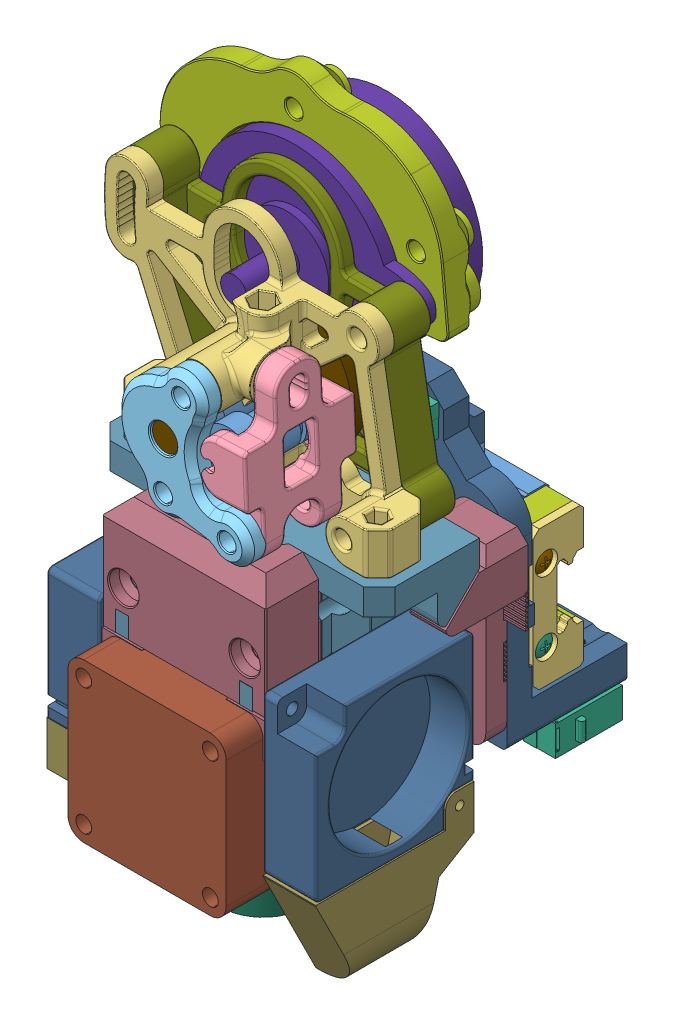
SolidWorks assembly TAP方案组装, configuration 默认. Lengths in mm.
Overall size (64.59 127.51 68).
53 component instances, 36 part files, 69 mates.
Components (placement in the parent):
- MGN12H (1)-1: MGN12H (1) [默认] at (-136.0725 0.7767 37.4) size (45.4 27 10)
  - PRODUCT_NAME_1 (1)^MGN12H (1)-1: PRODUCT_NAME_1 (1)^MGN12H (1) [默认] at origin size (32.4 27 10) (virtual)
  - PRODUCT_NAME_6 (1)^MGN12H (1)-1: PRODUCT_NAME_6 (1)^MGN12H (1) [默认] at origin size (1.59 4 4) (virtual)
  - PRODUCT_NAME_5 (1)^MGN12H (1)-1: PRODUCT_NAME_5 (1)^MGN12H (1) [默认] at origin size (1.5 26.4 9.6) (virtual)
  - PRODUCT_NAME_7 (1)^MGN12H (1)-1: PRODUCT_NAME_7 (1)^MGN12H (1) [默认] at origin size (1.59 4 4) (virtual)
  - PRODUCT_NAME_4 (1)^MGN12H (1)-1: PRODUCT_NAME_4 (1)^MGN12H (1) [默认] at origin size (1.5 26.4 9.6) (virtual)
  - PRODUCT_NAME_8 (1)^MGN12H (1)-1: PRODUCT_NAME_8 (1)^MGN12H (1) [默认] at origin size (1.59 4 4) (virtual)
  - PRODUCT_NAME_3 (1)^MGN12H (1)-1: PRODUCT_NAME_3 (1)^MGN12H (1) [默认] at origin size (5 26.4 9.6) (virtual)
  - PRODUCT_NAME_2 (1)^MGN12H (1)-1: PRODUCT_NAME_2 (1)^MGN12H (1) [默认] at origin size (5 26.4 9.6) (virtual)
  - PRODUCT_NAME_9 (1)^MGN12H (1)-1: PRODUCT_NAME_9 (1)^MGN12H (1) [默认] at origin size (1.59 4 4) (virtual)
- TAP方案底座-1: TAP方案底座 [默认] at (-18.5725 -19.2233 55.2) x (1 0 0) z (0 1 0) size (46 22.8 58)
- MGN9-6-2: MGN9-6 [默认] at (1.4275 238.2767 57.65) x (1 0 0) z (0 -1 0) size (9 6.5 50)
- MGN9H v1 v1-2: MGN9H v1 v1 [默认] at (-179.5291 -200.6019 -88.0682) x (0 0 1) z (-1 0 0) size (8 40.67 20)
- mini-V6固定座-1-1: mini-V6固定座-1 [Default] at (1.4275 10.3463 78.4) size (31 28 15.59)
- TAP-mini-V6固定座-1: TAP-mini-V6固定座 [Default] at (1.4275 10.3463 78.4) x (-1 0 0) z (0 0 -1) size (54 29 25.05)
- V6散热器-1: V6散热器 [Default] at (1.4275 13.3463 78.4) x (-0.047745 0 -0.99886) z (-0.99886 0 0.047745) size (22.3 59 22.3)
- 挤出机组装-1: 挤出机组装 [Default] at (-22.0931 89.3773 37.2926) x (1 0 0) z (0 -1 0) size (59.93 46.35 49.64)
  - 挤出机电机座-1: 挤出机电机座 [Default] at (-24.1653 27.1074 25.8748) size (56.72 7.01 44.47)
  - 36圆饼电机-1: 36圆饼电机 [Default] at (15.4554 9.6074 38.0093) x (0.99525 0 -0.097355) z (0.097355 0 0.99525) size (49.93 29 36.4)
  - BMG主齿组装-1: BMG主齿组装 [Default] at (16.3112 26.812 26.7681) x (0.995449 0 0.095298) z (-0.095298 0 0.995449) size (25.9 28.3 25.9)
    - BMG主齿-1: BMG主齿 [Default] at (5.4147 0.2954 24.6592) size (25.9 28.3 25.9)
    - BMG挤出齿-1: BMG挤出齿 [Default] at (5.4147 25.5954 24.6592) x (-0.887226 0 -0.461335) z (-0.461335 0 0.887226) size (9.4 14 9.4)
  - MR85-1: MR85 [Default] at (19.3513 27.6074 51.831) size (8 2.5 8)
  - 挤出机主体-1: 挤出机主体 [Default] at (-24.1653 34.1074 25.8748) size (59.44 18.3 40.97)
  - 挤出机从挤出齿轮支架-1: 挤出机从挤出齿轮支架 [Default] at (34.3823 55.9074 36.7653) x (0.043131 0 0.999069) z (0 -1 0) size (30 8.53 21.09)
  - BMG挤出齿-2: BMG挤出齿 [Default] at (28.0327 52.4074 51.9833) x (-0.837169 0 -0.546944) z (-0.546944 0 0.837169) size (9.4 14 9.4)
  - 挤出机盖子-1: 挤出机盖子 [Default] at (19.3513 55.9074 51.831) x (0.999977 0 0.006798) z (0.006798 0 -0.999977) size (25.23 3.5 27.46)
  - MR85-2: MR85 [Default] at (19.3513 54.9074 51.831) x (-0.837169 0 -0.546944) z (-0.546944 0 0.837169) size (8 2.5 8)
- KW10 Microswitch v1-1: KW10 Microswitch v1 [默认] at (-74.8225 32.1767 149.1) x (-1 0 0) z (0 -1 0) size (13.18 11.3 12.93)
  - M2x10 Self-tapping Screw (14) v1^KW10 Microswitch v1-1: M2x10 Self-tapping Screw (14) v1^KW10 Microswitch v1 [默认] at (-76.75 95.2 1.4) x (0 0 1) z (0 1 0) size (3.5 3.5 11.3) (hidden, virtual)
  - M2x10 Self-tapping Screw (14) v1 (1)^KW10 Microswitch v1-1: M2x10 Self-tapping Screw (14) v1 (1)^KW10 Microswitch v1 [默认] at (-83.25 95.2 1.4) x (0 0 1) z (0 1 0) size (3.5 3.5 11.3) (hidden, virtual)
  - KW10 Microswitch v1-3^KW10 Microswitch v1-1: KW10 Microswitch v1-3^KW10 Microswitch v1 [默认] at origin size (13.08 3.8 4.39) (hidden, virtual)
  - KW10 Microswitch v1-4^KW10 Microswitch v1-1: KW10 Microswitch v1-4^KW10 Microswitch v1 [默认] at origin size (12.8 5.8 10.15) (virtual)
- KW10 Microswitch v1-2: KW10 Microswitch v1 [默认] at (18.0275 -113.1233 -40.35) x (0 0 -1) z (1 0 0) size (13.18 11.3 12.93)
  - M2x10 Self-tapping Screw (14) v1^KW10 Microswitch v1-1: M2x10 Self-tapping Screw (14) v1^KW10 Microswitch v1 [默认] at (-76.75 95.2 1.4) x (0 0 1) z (0 1 0) size (3.5 3.5 11.3) (hidden, virtual)
  - M2x10 Self-tapping Screw (14) v1 (1)^KW10 Microswitch v1-1: M2x10 Self-tapping Screw (14) v1 (1)^KW10 Microswitch v1 [默认] at (-83.25 95.2 1.4) x (0 0 1) z (0 1 0) size (3.5 3.5 11.3) (hidden, virtual)
  - KW10 Microswitch v1-3^KW10 Microswitch v1-1: KW10 Microswitch v1-3^KW10 Microswitch v1 [默认] at origin size (13.08 3.8 4.39) (hidden, virtual)
  - KW10 Microswitch v1-4^KW10 Microswitch v1-1: KW10 Microswitch v1-4^KW10 Microswitch v1 [默认] at origin size (12.8 5.8 10.15) (virtual)
- head_pcb固定-1: head_pcb固定 [默认] at (17.7256 78.8706 62.4) x (0 0 -1) z (0.99525 0.097355 0) size (8 33 53.85)
- head_pcb固定-BIG-1: head_pcb固定-BIG [默认] at (14.1113 75.5027 46.4) x (0 0 -1) z (0.99525 0.097355 0) size (12 48.5 51.85) (hidden)
- 6x3磁铁-1: 6x3磁铁 [默认] at (-20.5725 14.4764 67.087) x (-0.617847 -0.555997 0.555997) z (-0.786299 0.436884 -0.436884) size (6 3 6)
- TAP皮带盖板-2: TAP皮带盖板 [默认] at (-21.5725 -17.2233 55.2) x (0 1 0) z (1 0 0) size (36 15.64 14)
- 6x3磁铁-2: 6x3磁铁 [默认] at (-20.5725 11.9684 65.2485) x (-0.369958 -0.656937 0.656937) z (-0.929049 0.2616 -0.2616) size (6 3 6)
- 3010涡轮-1: 3010涡轮 [Default] at (-14.0725 6.171 63.9058) x (0 0 1) z (0 -1 0) size (30 10.07 30)
- 3010风扇-1: 3010风扇 [Default] at (-13.5725 0.9463 90.4) x (1 0 0) z (0 -1 0) size (30 10 30)
- 3010涡轮适配-短-1: 3010涡轮适配-短 [默认] at (-12.0725 -18.079 63.9058) x (0 0 1) z (0 -1 0) size (30.03 10 25.6)
- 3010涡轮-2: 3010涡轮 [Default] at (16.9275 6.171 93.9058) x (0 0 -1) z (0 -1 0) size (30 10.07 30)
- 3010涡轮适配-短-2: 3010涡轮适配-短 [默认] at (14.9275 -18.079 93.9058) x (0 0 -1) z (0 -1 0) size (30.03 10 25.6)
- 镜向TAP皮带盖板-6: 镜向TAP皮带盖板 [默认] at (24.4275 -17.2233 55.2) x (0 1 0) z (1 0 0) size (36 15.64 14)
- 吹料风扇螺母-1: 吹料风扇螺母 [默认] at (14.4275 1.4463 93.45) x (0 1 0) z (-1 0 0) size (3.92 4.5 2.4)
- 吹料风扇螺母-2: 吹料风扇螺母 [默认] at (-9.1725 1.4463 93.35) x (0 1 0) z (-1 0 0) size (3.92 4.5 2.4)
- 吹料风扇螺母-3: 吹料风扇螺母 [默认] at (14.4275 5.3663 64.35) x (0 -1 0) z (-1 0 0) size (3.92 4.5 2.4)
- 吹料风扇螺母-4: 吹料风扇螺母 [默认] at (-11.5725 1.4463 64.35) x (0 1 0) z (1 0 0) size (3.92 4.5 2.4)
Mates (geometry in assembly coordinates):
- 同心3: concentric aligned: circle of MGN12H (1)-1/PRODUCT_NAME_1 (1)^MGN12H (1)-1; circle of TAP方案底座-1
- 同心4: concentric aligned: circle of MGN12H (1)-1/PRODUCT_NAME_1 (1)^MGN12H (1)-1; circle of TAP方案底座-1
- 重合5: coincident anti-aligned: plane of MGN12H (1)-1/PRODUCT_NAME_1 (1)^MGN12H (1)-1 through (-14.7725 0.7767 50) normal (0 0 1); plane of TAP方案底座-1 through (-18.5725 -19.2233 50) normal (0 0 -1)
- 重合7: coincident anti-aligned: plane of MGN9-6-2 through (-2.8725 -11.7233 60.9) normal (0 0 1); plane of MGN9H v1 v1-2 through (1.4275 19.3963 60.9) normal (0 0 -1)
- 重合8: coincident anti-aligned: plane of MGN9-6-2 through (-3.0725 -11.7233 54.6) normal (-1 0 0); plane of MGN9H v1 v1-2 through (-3.0725 19.3963 60.4) normal (1 0 0)
- 同心8: concentric aligned: circle of TAP方案底座-1; circle of MGN9-6-2
- 同心9: concentric aligned: circle of TAP方案底座-1; circle of MGN9-6-2
- 重合9: coincident anti-aligned: plane of TAP方案底座-1 through (-18.5725 -19.2233 54.4) normal (0 0 1); plane of MGN9-6-2 through (-2.8725 -11.7233 54.4) normal (0 0 -1)
- 同心12: concentric aligned: cylinder of TAP-mini-V6固定座-1 through (1.4275 4.4463 78.4) axis (0 1 0) radius 6.05; cylinder of V6散热器-1 through (1.4275 4.3463 78.4) axis (0 1 0) radius 6
- 重合17: coincident anti-aligned: plane of TAP-mini-V6固定座-1 through (1.4275 10.3463 78.4) normal (0 1 0); plane of V6散热器-1 through (1.4275 10.3463 78.4) normal (0 -1 0)
- 重合18: coincident anti-aligned: plane of MGN9H v1 v1-2 through (1.4275 19.3963 64.4) normal (0 0 1); plane of TAP-mini-V6固定座-1 through (1.4275 10.3463 64.4) normal (0 0 -1)
- 重合19: coincident anti-aligned: plane of TAP-mini-V6固定座-1 through (1.4275 22.4463 78.4) normal (0 1 0); plane of 挤出机组装-1/挤出机主体-1 through (-46.2583 22.4463 74.4) normal (0 -1 0)
- 锁定1: lock: unknown of TAP-mini-V6固定座-1; unknown of 挤出机组装-1/挤出机主体-1
- 同心14: concentric anti-aligned: cylinder of MGN9H v1 v1-2 through (-6.0725 12.4463 61.4) axis (0 0 1) radius 1.5; cylinder of TAP-mini-V6固定座-1 through (-6.0725 12.4463 89.45) axis (0 0 -1) radius 1.6
- 同心15: concentric aligned: circle of MGN9H v1 v1-2; cylinder of TAP-mini-V6固定座-1 through (8.9275 -3.5537 89.45) axis (0 0 -1) radius 1.6
- 同心17: concentric aligned: cylinder of TAP-mini-V6固定座-1 through (-6.0725 -3.5537 66.9) axis (0 0 1) radius 2.9; cylinder of 复件 M3x12 BHCS v1 (1) (1) (1)-1 through (-6.0725 -3.7824 60.6812) axis (0 0 1) radius 1.5
- 重合22: coincident anti-aligned: plane of TAP-mini-V6固定座-1 through (-6.0725 -3.5537 66.9) normal (0 0 1); plane of 复件 M3x12 BHCS v1 (1) (1) (1)-1 through (-4.9542 -6.4039 66.9) normal (0 0 -1)
- 同心18: concentric anti-aligned: cylinder of TAP-mini-V6固定座-1 through (-6.0725 12.4463 89.45) axis (0 0 -1) radius 1.6; cylinder of 复件 M3x12 BHCS v1 (1) (1) (1)-2 through (-6.0725 12.2176 65.0812) axis (0 0 1) radius 1.5
- 重合23: coincident anti-aligned: plane of TAP-mini-V6固定座-1 through (-6.0725 12.4463 71.3) normal (0 0 1); plane of 复件 M3x12 BHCS v1 (1) (1) (1)-2 through (-8.3035 10.4442 71.3) normal (0 0 -1)
- 同心19: concentric anti-aligned: cylinder of mini-V6固定座-1-1 through (1.4275 17.4463 78.4) axis (0 1 0) radius 11.05; cylinder of TAP-mini-V6固定座-1 through (1.4275 17.4463 78.4) axis (0 -1 0) radius 11.05
- 重合24: coincident aligned: plane of mini-V6固定座-1-1 through (1.4275 22.4463 78.4) normal (0 1 0); plane of TAP-mini-V6固定座-1 through (1.4275 22.4463 78.4) normal (0 1 0)
- 重合25: coincident anti-aligned: plane of TAP方案底座-1 through (-18.5725 -19.2233 55.2) normal (0 0 1); plane of KW10 Microswitch v1-1/KW10 Microswitch v1-4^KW10 Microswitch v1-1 through (-1.2225 32.2767 55.2) normal (0 0 -1)
- 锁定2: lock: unknown of TAP-mini-V6固定座-1; unknown of 挤出机组装-1/挤出机主体-1
- 重合30: coincident anti-aligned: plane of TAP方案底座-1 through (-18.5725 -19.2233 50.4) normal (0 -1 0); plane of KW10 Microswitch v1-2/KW10 Microswitch v1-4^KW10 Microswitch v1-1 through (17.9275 -19.2233 33.25) normal (0 1 0)
- 锁定5: lock: unknown of TAP方案底座-1; unknown of KW10 Microswitch v1-2/KW10 Microswitch v1-4^KW10 Microswitch v1-1
- 锁定6: lock: unknown of TAP方案底座-1; unknown of KW10 Microswitch v1-2/KW10 Microswitch v1-4^KW10 Microswitch v1-1
- 同心29: concentric aligned: cylinder of 挤出机组装-1/36圆饼电机-1 through (-28.4585 49.2335 62.4) axis (0 0 1) radius 1.5; cylinder of head_pcb固定-1 through (-28.4585 49.2335 58.4) axis (0 0 1) radius 1.6
- 同心30: concentric aligned: cylinder of 挤出机组装-1/36圆饼电机-1 through (15.1832 53.5026 62.4) axis (0 0 1) radius 1.5; cylinder of head_pcb固定-1 through (15.1832 53.5026 58.4) axis (0 0 1) radius 1.6
- 重合34: coincident anti-aligned: plane of 挤出机组装-1/36圆饼电机-1 through (-6.6377 51.3681 62.4) normal (0 0 -1); plane of head_pcb固定-1 through (17.7256 78.8706 62.4) normal (0 0 1)
- 同心39: concentric anti-aligned: cylinder of head_pcb固定-1 through (14.4044 61.4646 54.4) axis (0 0 1) radius 3; cylinder of head_pcb固定-BIG-1 through (14.4044 61.4646 54.4) axis (0 0 -1) radius 3
- 同心40: concentric anti-aligned: cylinder of head_pcb固定-1 through (-8.7795 73.2636 54.4) axis (0 0 1) radius 3; cylinder of head_pcb固定-BIG-1 through (-8.7795 73.2636 54.4) axis (0 0 -1) radius 3
- 重合38: coincident anti-aligned: plane of head_pcb固定-1 through (14.4044 61.4646 54.4) normal (0 0 -1); plane of head_pcb固定-BIG-1 through (14.4044 61.4646 54.4) normal (0 0 1)
- 距离1: distance = 0 mm anti-aligned: plane of TAP方案底座-1 through (-18.5725 -19.2233 55.2) normal (0 0 1); plane of TAP皮带盖板-2 through (-21.5725 -17.2233 55.2) normal (0 0 -1)
- 同心41: concentric aligned: cylinder of TAP方案底座-1 through (-16.5725 11.7767 60.4) axis (0 0 -1) radius 1.6; cylinder of TAP皮带盖板-2 through (-16.5725 11.7767 59.2) axis (0 0 -1) radius 1.6
- 同心42: concentric aligned: cylinder of TAP方案底座-1 through (-16.5725 -10.2233 60.4) axis (0 0 -1) radius 1.6; cylinder of TAP皮带盖板-2 through (-16.5725 -10.2233 59.2) axis (0 0 -1) radius 1.6
- 同心44: concentric aligned: cylinder of TAP-mini-V6固定座-1 through (-20.5725 16.5978 69.2083) axis (0 -0.707107 -0.707107) radius 3.1; cylinder of 6x3磁铁-1 through (-20.5725 16.5978 69.2083) axis (0 -0.707107 -0.707107) radius 3
- 重合44: coincident anti-aligned: plane of TAP-mini-V6固定座-1 through (-20.5725 16.5978 69.2083) normal (0 -0.707107 -0.707107); plane of 6x3磁铁-1 through (-20.5725 16.5978 69.2083) normal (0 0.707107 0.707107)
- 同心45: concentric anti-aligned: cylinder of TAP皮带盖板-2 through (-20.5725 11.9684 65.2485) axis (0 0.707107 0.707107) radius 3.1; cylinder of 6x3磁铁-2 through (-20.5725 14.0897 67.3698) axis (0 -0.707107 -0.707107) radius 3
- 重合45: coincident anti-aligned: plane of TAP皮带盖板-2 through (-20.5725 11.9684 65.2485) normal (0 0.707107 0.707107); plane of 6x3磁铁-2 through (-20.5725 11.9684 65.2485) normal (0 -0.707107 -0.707107)
- 平行2: parallel aligned: plane of mini-V6固定座-1-1 through (-14.0725 -5.5537 83.4) normal (0 0 -1); plane of TAP-mini-V6固定座-1 through (1.4275 10.3463 64.4) normal (0 0 -1)
- 重合51: coincident anti-aligned: plane of mini-V6固定座-1-1 through (1.4275 10.3463 90.4) normal (0 0 1); plane of 3010风扇-1 through (-13.5725 0.9463 90.4) normal (0 0 -1)
- 同心47: concentric aligned: cylinder of mini-V6固定座-1-1 through (13.4275 -2.0537 83.4) axis (0 0 1) radius 1.45; cylinder of 3010风扇-1 through (13.4275 -2.0537 90.4) axis (0 0 1) radius 1.5
- 同心48: concentric aligned: cylinder of mini-V6固定座-1-1 through (-10.5725 -2.0537 83.4) axis (0 0 1) radius 1.45; cylinder of 3010风扇-1 through (-10.5725 -2.0537 90.4) axis (0 0 1) radius 1.5
- 同心49: concentric anti-aligned: cylinder of 3010涡轮-1 through (-14.0725 -21.079 91.1558) axis (-1 0 0) radius 1.1; cylinder of 3010涡轮适配-短-1 through (-24.0725 -21.079 91.1558) axis (1 0 0) radius 0.8
- 平行4: parallel anti-aligned: plane of 3010涡轮-1 through (-24.0725 -23.829 63.9058) normal (0 -1 0); plane of 3010涡轮适配-短-1 through (-24.0725 -23.879 63.9058) normal (0 1 0)
- 重合53: coincident aligned: plane of 3010涡轮-1 through (-24.0725 6.171 63.9058) normal (-1 0 0); plane of 3010涡轮适配-短-1 through (-24.0725 -18.079 63.9058) normal (-1 0 0)
- 重合55: coincident anti-aligned: plane of mini-V6固定座-1-1 through (-14.0725 -5.5537 83.4) normal (-1 0 0); plane of 3010涡轮-1 through (-14.0725 6.171 63.9058) normal (1 0 0)
- 平行5: parallel anti-aligned: plane of mini-V6固定座-1-1 through (1.4275 -5.5537 78.4) normal (0 -1 0); plane of 3010涡轮-1 through (-24.0725 6.171 63.9058) normal (0 1 0)
- 同心51: concentric anti-aligned: cylinder of 3010涡轮-2 through (16.9275 -21.079 66.6558) axis (1 0 0) radius 1.1; cylinder of 3010涡轮适配-短-2 through (26.9275 -21.079 66.6558) axis (-1 0 0) radius 0.8
- 重合57: coincident aligned: plane of 3010涡轮-2 through (26.9275 6.171 93.9058) normal (1 0 0); plane of 3010涡轮适配-短-2 through (26.9275 -18.079 93.9058) normal (1 0 0)
- 平行6: parallel anti-aligned: plane of 3010涡轮-2 through (26.9275 -23.829 93.9058) normal (0 -1 0); plane of 3010涡轮适配-短-2 through (26.9275 -23.879 93.9058) normal (0 1 0)
- 重合58: coincident anti-aligned: plane of mini-V6固定座-1-1 through (16.9275 -5.5537 83.4) normal (1 0 0); plane of 3010涡轮-2 through (16.9275 6.171 93.9058) normal (-1 0 0)
- 重合59: coincident aligned: plane of 3010涡轮-1 through (-24.0725 6.171 93.9058) normal (0 0 1); plane of 3010涡轮-2 through (26.9275 6.171 93.9058) normal (0 0 1)
- 重合60: coincident aligned: plane of 3010涡轮-1 through (-24.0725 6.171 63.9058) normal (0 1 0); plane of 3010涡轮-2 through (26.9275 6.171 93.9058) normal (0 1 0)
- 锁定4: lock: unknown of TAP-mini-V6固定座-1; unknown of 3010涡轮-1
- 重合61: coincident anti-aligned: plane of mini-V6固定座-1-1 through (11.9275 5.3663 88.9) normal (0 -1 0); plane of 吹料风扇螺母-1 through (14.4275 5.3663 88.95) normal (0 1 0)
- 重合63: coincident anti-aligned: plane of mini-V6固定座-1-1 through (14.4275 5.3663 88.9) normal (-1 0 0); plane of 吹料风扇螺母-1 through (14.4275 1.4463 88.95) normal (1 0 0)
- 重合65: coincident anti-aligned: plane of mini-V6固定座-1-1 through (-9.0725 5.3663 88.9) normal (0 -1 0); plane of 吹料风扇螺母-2 through (-9.1725 5.3663 88.85) normal (0 1 0)
- 重合66: coincident anti-aligned: plane of mini-V6固定座-1-1 through (-9.0725 10.3463 90.15) normal (-0.707107 0 0.707107); plane of 吹料风扇螺母-2 through (-10.3725 1.4463 88.85) normal (0.707107 0 -0.707107)
- 重合67: coincident anti-aligned: plane of mini-V6固定座-1-1 through (-11.5725 5.3663 88.9) normal (1 0 0); plane of 吹料风扇螺母-2 through (-11.5725 1.4463 88.85) normal (-1 0 0)
- 重合68: coincident anti-aligned: plane of TAP-mini-V6固定座-1 through (11.9275 1.4463 68.9) normal (0 1 0); plane of 吹料风扇螺母-3 through (14.4275 1.4463 68.85) normal (0 -1 0)
- 重合69: coincident anti-aligned: plane of TAP-mini-V6固定座-1 through (14.4275 5.4463 67.65) normal (-0.707107 0 -0.707107); plane of 吹料风扇螺母-3 through (13.2275 5.3663 68.85) normal (0.707107 0 0.707107)
- 重合70: coincident anti-aligned: plane of TAP-mini-V6固定座-1 through (14.4275 5.4463 68.9) normal (-1 0 0); plane of 吹料风扇螺母-3 through (14.4275 5.3663 68.85) normal (1 0 0)
- 重合71: coincident anti-aligned: plane of TAP-mini-V6固定座-1 through (-9.0725 1.4463 68.9) normal (0 1 0); plane of 吹料风扇螺母-4 through (-11.5725 1.4463 68.85) normal (0 -1 0)
- 重合72: coincident anti-aligned: plane of TAP-mini-V6固定座-1 through (-10.3225 10.3463 68.9) normal (0.707107 0 -0.707107); plane of 吹料风扇螺母-4 through (-10.3725 1.4463 68.85) normal (-0.707107 0 0.707107)
- 重合73: coincident anti-aligned: plane of TAP-mini-V6固定座-1 through (-11.5725 5.4463 68.9) normal (1 0 0); plane of 吹料风扇螺母-4 through (-11.5725 1.4463 68.85) normal (-1 0 0)
- 重合75: coincident anti-aligned: plane of mini-V6固定座-1-1 through (13.1775 10.3463 88.9) normal (-0.707107 0 0.707107); plane of 吹料风扇螺母-1 through (13.2275 1.4463 88.95) normal (0.707107 0 -0.707107)
- 同心52: concentric anti-aligned: cylinder of TAP方案底座-1 through (1.9275 30.7767 46.4) axis (0 0 1) radius 0.9; circle of KW10 Microswitch v1-1/KW10 Microswitch v1-4^KW10 Microswitch v1-1
- 同心53: concentric anti-aligned: circle of TAP方案底座-1; circle of KW10 Microswitch v1-1/KW10 Microswitch v1-4^KW10 Microswitch v1-1
